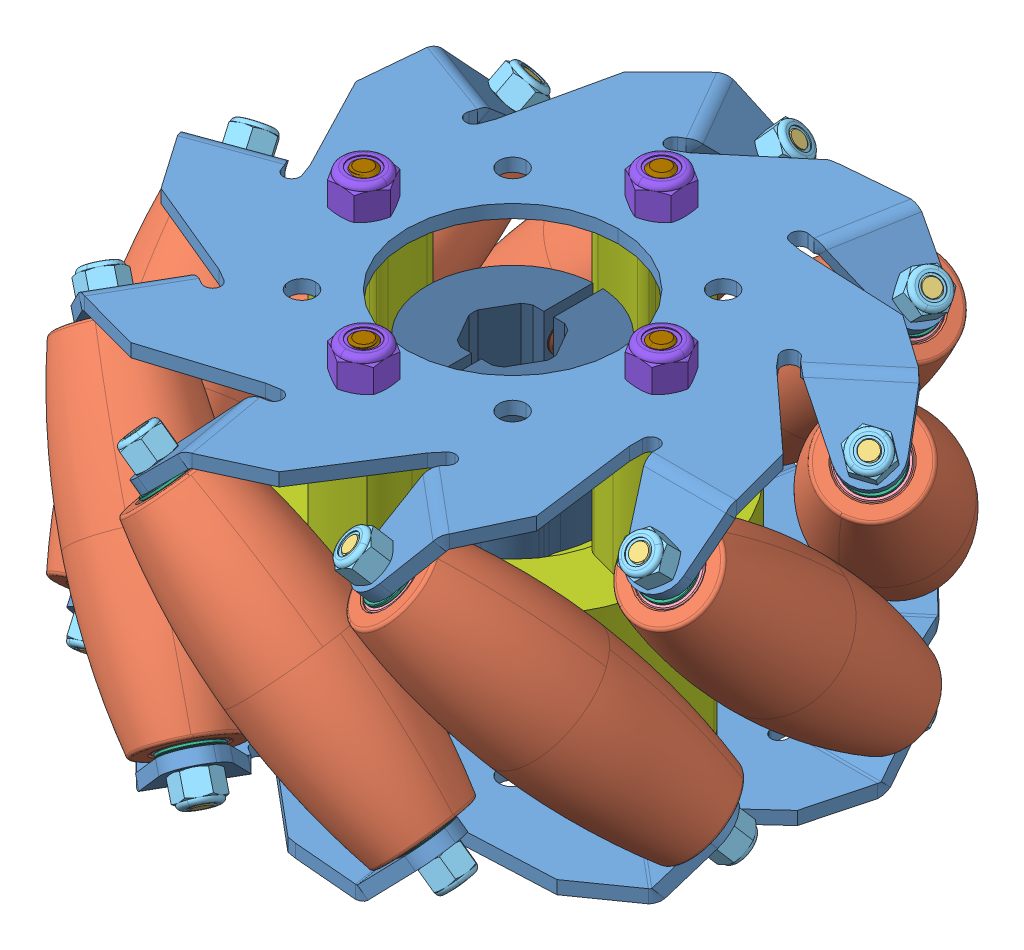
SolidWorks assembly Mecanum Right Slant With Hyper Hub, configuration Default. Lengths in mm.
Overall size (118.19 59.77 119.24).
88 component instances, 11 part files, 0 mates.
Components (placement in the parent):
- Mecanum 1.STEP-1: Mecanum 1.STEP [Default] at origin size (118.19 59.77 119.24)
  - 3606-0100-0100 Side Plate.STEP-1: 3606-0100-0100 Side Plate.STEP [Default] at (-29.0217 8.9207 26.0563) size (93.83 10.59 94.33)
  - 3606-0100-0100 Side Plate.STEP-2: 3606-0100-0100 Side Plate.STEP [Default] at (-29.0217 -77.2207 26.0563) x (1 0 0) z (0 0 -1) size (93.83 10.59 94.33)
  - 3606-XXXX-0100 Hi Durability Roller.STEP-1: 3606-XXXX-0100 Hi Durability Roller.STEP [Default] at (21.1711 -21.7418 81.2623) x (0.224554 0.052172 0.973064) z (0.696364 -0.707107 -0.122788) size (28.35 23.77 47)
  - 3606-XXXX-0100 Roller Axle.STEP-1: 3606-XXXX-0100 Roller Axle.STEP [Default] at (-21.9538 -34.2162 65.7074) x (0.715939 0.696364 0.050088) z (0.050088 -0.122788 0.991168) size (4 60.01 4)
  - 3606-XXXX-0100 Roller Bearing.STEP-1: 3606-XXXX-0100 Roller Bearing.STEP [Default] at (-35.5329 -20.4276 68.1018) x (0.715939 0.696364 0.050088) z (0.050088 -0.122788 0.991168) size (9 4 9)
  - 3606-XXXX-0100 Roller Locknut_90576A102.STEP-1: 3606-XXXX-0100 Roller Locknut_90576A102.STEP [Default] at (-40.1289 -15.7607 68.9122) x (0.353014 0.486435 -0.799226) z (0.624866 0.513207 0.588354) size (5.52 4.01 6.37)
  - 3606-XXXX-0100 Roller Shim.STEP-1: 3606-XXXX-0100 Roller Shim.STEP [Default] at (18.11 -15.3241 52.0807) x (0.434371 0.830389 -0.348965) z (-0.303693 0.499753 0.811183) size (7.84 5.87 6.18)
  - 3606-XXXX-0100 Wheel Center.STEP-1: 3606-XXXX-0100 Wheel Center.STEP [Default] at (-29.0217 -34.15 26.0563) x (-0.707107 0 0.707107) z (-0.707107 0 -0.707107) size (54 46 54)
  - 3606-XXXX-0100 Roller Bearing.STEP-2: 3606-XXXX-0100 Roller Bearing.STEP [Default] at (-8.514 -47.8634 63.3376) x (0.715939 0.696364 0.050088) z (-0.050088 0.122788 -0.991168) size (9 4 9)
  - 3606-XXXX-0100 Roller Shim.STEP-2: 3606-XXXX-0100 Roller Shim.STEP [Default] at (-6.4986 -109.4838 69.5446) x (-0.771195 -0.488369 0.408356) z (-0.621724 0.439939 -0.648007) size (7.84 5.87 6.18)
  - 3606-XXXX-0100 Roller Locknut_90576A102.STEP-2: 3606-XXXX-0100 Roller Locknut_90576A102.STEP [Default] at (-3.918 -52.5303 62.5272) x (-0.353014 -0.486435 0.799226) z (0.624866 0.513207 0.588354) size (5.52 4.01 6.37)
  - 3606-XXXX-0100 Roller Locknut_90576A102.STEP-3: 3606-XXXX-0100 Roller Locknut_90576A102.STEP [Default] at (-65.0776 -15.7607 51.7463) x (0.784157 0.486435 -0.38533) z (0.100489 0.513207 0.852362) size (5.52 4.01 6.37)
  - 3606-XXXX-0100 Roller Locknut_90576A102.STEP-4: 3606-XXXX-0100 Roller Locknut_90576A102.STEP [Default] at (-73.1553 -15.7607 22.5597) x (0.848384 0.486435 0.208867) z (-0.470909 0.513207 0.71754) size (5.52 4.01 6.37)
  - 3606-XXXX-0100 Roller Locknut_90576A102.STEP-5: 3606-XXXX-0100 Roller Locknut_90576A102.STEP [Default] at (-60.5824 -15.7607 -4.9907) x (0.515643 0.486435 0.705332) z (-0.821963 0.513207 0.246973) size (5.52 4.01 6.37)
  - 3606-XXXX-0100 Roller Locknut_90576A102.STEP-6: 3606-XXXX-0100 Roller Locknut_90576A102.STEP [Default] at (-33.242 -15.7607 -18.0139) x (-0.058373 0.486435 0.871765) z (-0.788411 0.513207 -0.339155) size (5.52 4.01 6.37)
  - 3606-XXXX-0100 Roller Locknut_90576A102.STEP-7: 3606-XXXX-0100 Roller Locknut_90576A102.STEP [Default] at (-3.9268 -15.7607 -10.4161) x (-0.605076 0.486435 0.630289) z (-0.385953 0.513207 -0.766589) size (5.52 4.01 6.37)
  - 3606-XXXX-0100 Roller Locknut_90576A102.STEP-8: 3606-XXXX-0100 Roller Locknut_90576A102.STEP [Default] at (13.6461 -15.7607 14.2475) x (-0.868657 0.486435 0.093894) z (0.197097 0.513207 -0.835327) size (5.52 4.01 6.37)
  - 3606-XXXX-0100 Roller Locknut_90576A102.STEP-9: 3606-XXXX-0100 Roller Locknut_90576A102.STEP [Default] at (11.2543 -15.7607 44.4366) x (-0.725784 0.486435 -0.486435) z (0.687923 0.513207 -0.513207) size (5.52 4.01 6.37)
  - 3606-XXXX-0100 Roller Locknut_90576A102.STEP-10: 3606-XXXX-0100 Roller Locknut_90576A102.STEP [Default] at (-9.9831 -15.7607 66.0254) x (-0.243308 0.486435 -0.839156) z (0.856862 0.513207 0.049049) size (5.52 4.01 6.37)
  - 3606-XXXX-0100 Roller Shim.STEP-3: 3606-XXXX-0100 Roller Shim.STEP [Default] at (-9.6449 -15.3241 76.2879) x (0.557058 0.830389 0.011885) z (-0.75406 0.499753 0.426192) size (7.84 5.87 6.18)
  - 3606-XXXX-0100 Roller Shim.STEP-4: 3606-XXXX-0100 Roller Shim.STEP [Default] at (-46.4664 -15.3241 76.9911) x (0.419091 0.830389 0.367174) z (-0.851595 0.499753 -0.158218) size (7.84 5.87 6.18)
  - 3606-XXXX-0100 Roller Shim.STEP-5: 3606-XXXX-0100 Roller Shim.STEP [Default] at (-75.1254 -15.3241 53.8614) x (0.085028 0.830389 0.550659) z (-0.550659 0.499753 -0.668597) size (7.84 5.87 6.18)
  - 3606-XXXX-0100 Roller Shim.STEP-6: 3606-XXXX-0100 Roller Shim.STEP [Default] at (-82.2119 -15.3241 17.7214) x (-0.288822 0.830389 0.476484) z (0.007937 0.499753 -0.866131) size (7.84 5.87 6.18)
  - 3606-XXXX-0100 Roller Shim.STEP-7: 3606-XXXX-0100 Roller Shim.STEP [Default] at (-64.4102 -15.3241 -14.5186) x (-0.527528 0.830389 0.179357) z (0.562818 0.499753 -0.658393) size (7.84 5.87 6.18)
  - 3606-XXXX-0100 Roller Shim.STEP-8: 3606-XXXX-0100 Roller Shim.STEP [Default] at (-30.0498 -15.3241 -27.7731) x (-0.519398 0.830389 -0.201693) z (0.854351 0.499753 -0.142586) size (7.84 5.87 6.18)
  - 3606-XXXX-0100 Roller Shim.STEP-9: 3606-XXXX-0100 Roller Shim.STEP [Default] at (4.7916 -15.3241 -15.8403) x (-0.268236 0.830389 -0.488369) z (0.746123 0.499753 0.439939) size (7.84 5.87 6.18)
  - 3606-XXXX-0100 Roller Shim.STEP-10: 3606-XXXX-0100 Roller Shim.STEP [Default] at (23.8114 -15.3241 15.6965) x (0.108437 0.830389 -0.546531) z (0.288776 0.499753 0.816612) size (7.84 5.87 6.18)
  - 3606-XXXX-0100 Roller Bearing.STEP-3: 3606-XXXX-0100 Roller Bearing.STEP [Default] at (-61.0359 -20.4276 54.0797) x (0.516245 0.696364 0.498566) z (-0.598741 -0.122788 0.791475) size (9 4 9)
  - 3606-XXXX-0100 Roller Bearing.STEP-4: 3606-XXXX-0100 Roller Bearing.STEP [Default] at (-71.5591 -20.4276 26.9452) x (0.074995 0.696364 0.71376) z (-0.967412 -0.122788 0.221441) size (9 4 9)
  - 3606-XXXX-0100 Roller Bearing.STEP-5: 3606-XXXX-0100 Roller Bearing.STEP [Default] at (-62.1786 -20.4276 -0.6053) x (-0.401347 0.696364 0.594977) z (-0.883421 -0.122788 -0.452207) size (9 4 9)
  - 3606-XXXX-0100 Roller Bearing.STEP-6: 3606-XXXX-0100 Roller Bearing.STEP [Default] at (-37.2836 -20.4276 -15.6804) x (-0.689893 0.696364 0.197798) z (-0.386067 -0.122788 -0.914262) size (9 4 9)
  - 3606-XXXX-0100 Roller Bearing.STEP-7: 3606-XXXX-0100 Roller Bearing.STEP [Default] at (-8.5228 -20.4276 -11.2265) x (-0.655631 0.696364 -0.291932) z (0.291932 -0.122788 -0.948524) size (9 4 9)
  - 3606-XXXX-0100 Roller Bearing.STEP-8: 3606-XXXX-0100 Roller Bearing.STEP [Default] at (10.6463 -20.4276 10.6724) x (-0.314592 0.696364 -0.645065) z (0.833333 -0.122788 -0.538961) size (9 4 9)
  - 3606-XXXX-0100 Roller Bearing.STEP-9: 3606-XXXX-0100 Roller Bearing.STEP [Default] at (11.2543 -20.4276 39.7697) x (0.173648 0.696364 -0.696364) z (0.984808 -0.122788 0.122788) size (9 4 9)
  - 3606-XXXX-0100 Roller Bearing.STEP-10: 3606-XXXX-0100 Roller Bearing.STEP [Default] at (-6.9833 -20.4276 62.4503) x (0.580637 0.696364 -0.421827) z (0.67548 -0.122788 0.727083) size (9 4 9)
  - 3606-XXXX-0100 Hi Durability Roller.STEP-2: 3606-XXXX-0100 Hi Durability Roller.STEP [Default] at (-26.0575 -21.7418 100.6099) x (-0.453455 0.052172 0.889751) z (0.612372 -0.707107 0.353553) size (28.35 23.77 47)
  - 3606-XXXX-0100 Hi Durability Roller.STEP-3: 3606-XXXX-0100 Hi Durability Roller.STEP [Default] at (-74.6731 -21.7418 85.073) x (-0.919288 0.052172 0.390113) z (0.241845 -0.707107 0.664463) size (28.35 23.77 47)
  - 3606-XXXX-0100 Hi Durability Roller.STEP-4: 3606-XXXX-0100 Hi Durability Roller.STEP [Default] at (-101.9279 -21.7418 41.9216) x (-0.954975 0.052172 -0.292062) z (-0.241845 -0.707107 0.664463) size (28.35 23.77 47)
  - 3606-XXXX-0100 Hi Durability Roller.STEP-5: 3606-XXXX-0100 Hi Durability Roller.STEP [Default] at (-95.0691 -21.7418 -8.6533) x (-0.543819 0.052172 -0.837579) z (-0.612372 -0.707107 0.353553) size (28.35 23.77 47)
  - 3606-XXXX-0100 Hi Durability Roller.STEP-6: 3606-XXXX-0100 Hi Durability Roller.STEP [Default] at (-57.306 -21.7418 -42.9873) x (0.121796 0.052172 -0.991183) z (-0.696364 -0.707107 -0.122788) size (28.35 23.77 47)
  - 3606-XXXX-0100 Hi Durability Roller.STEP-7: 3606-XXXX-0100 Hi Durability Roller.STEP [Default] at (-6.3084 -21.7418 -45.0149) x (0.730421 0.052172 -0.681002) z (-0.454519 -0.707107 -0.541675) size (28.35 23.77 47)
  - 3606-XXXX-0100 Hi Durability Roller.STEP-8: 3606-XXXX-0100 Hi Durability Roller.STEP [Default] at (34.0614 -21.7418 -13.7876) x (0.997274 0.052172 -0.052172) z (0 -0.707107 -0.707107) size (28.35 23.77 47)
  - 3606-XXXX-0100 Hi Durability Roller.STEP-9: 3606-XXXX-0100 Hi Durability Roller.STEP [Default] at (44.9139 -21.7418 36.0832) x (0.797492 0.052172 0.60107) z (0.454519 -0.707107 -0.541675) size (28.35 23.77 47)
  - 3606-XXXX-0100 Roller Bearing.STEP-11: 3606-XXXX-0100 Roller Bearing.STEP [Default] at (-37.2758 -47.8634 67.7976) x (0.516245 0.696364 0.498566) z (0.598741 0.122788 -0.791475) size (9 4 9)
  - 3606-XXXX-0100 Roller Bearing.STEP-12: 3606-XXXX-0100 Roller Bearing.STEP [Default] at (-62.1755 -47.8634 52.7264) x (0.074995 0.696364 0.71376) z (0.967412 0.122788 -0.221441) size (9 4 9)
  - 3606-XXXX-0100 Roller Bearing.STEP-13: 3606-XXXX-0100 Roller Bearing.STEP [Default] at (-71.5622 -47.8634 25.1759) x (-0.401347 0.696364 0.594977) z (0.883421 0.122788 0.452207) size (9 4 9)
  - 3606-XXXX-0100 Roller Bearing.STEP-14: 3606-XXXX-0100 Roller Bearing.STEP [Default] at (-61.0437 -47.8634 -1.9626) x (-0.689893 0.696364 0.197798) z (0.386067 0.122788 0.914262) size (9 4 9)
  - 3606-XXXX-0100 Roller Bearing.STEP-15: 3606-XXXX-0100 Roller Bearing.STEP [Default] at (-35.5418 -47.8634 -15.9907) x (-0.655631 0.696364 -0.291932) z (-0.291932 0.122788 0.948524) size (9 4 9)
  - 3606-XXXX-0100 Roller Bearing.STEP-16: 3606-XXXX-0100 Roller Bearing.STEP [Default] at (-6.989 -47.8634 -10.3446) x (-0.314592 0.696364 -0.645065) z (-0.833333 0.122788 0.538961) size (9 4 9)
  - 3606-XXXX-0100 Roller Bearing.STEP-17: 3606-XXXX-0100 Roller Bearing.STEP [Default] at (11.2543 -47.8634 12.334) x (0.173648 0.696364 -0.696364) z (-0.984808 0.122788 -0.122788) size (9 4 9)
  - 3606-XXXX-0100 Roller Bearing.STEP-18: 3606-XXXX-0100 Roller Bearing.STEP [Default] at (10.6521 -47.8634 41.4333) x (0.580637 0.696364 -0.421827) z (-0.67548 0.122788 -0.727083) size (9 4 9)
  - 3606-XXXX-0100 Roller Shim.STEP-11: 3606-XXXX-0100 Roller Shim.STEP [Default] at (-39.7217 -109.4838 73.8479) x (-0.853256 -0.488369 -0.182895) z (-0.059738 0.439939 -0.896038) size (7.84 5.87 6.18)
  - 3606-XXXX-0100 Roller Shim.STEP-12: 3606-XXXX-0100 Roller Shim.STEP [Default] at (-67.9382 -109.4838 55.789) x (-0.536069 -0.488369 -0.688568) z (0.530201 0.439939 -0.724804) size (7.84 5.87 6.18)
  - 3606-XXXX-0100 Roller Shim.STEP-13: 3606-XXXX-0100 Roller Shim.STEP [Default] at (-77.9453 -109.4838 23.8178) x (0.03195 -0.488369 -0.872052) z (0.872052 0.439939 -0.214425) size (7.84 5.87 6.18)
  - 3606-XXXX-0100 Roller Shim.STEP-14: 3606-XXXX-0100 Roller Shim.STEP [Default] at (-65.0604 -109.4838 -7.1059) x (0.58502 -0.488369 -0.647494) z (0.805861 0.439939 0.396285) size (7.84 5.87 6.18)
  - 3606-XXXX-0100 Roller Shim.STEP-15: 3606-XXXX-0100 Roller Shim.STEP [Default] at (-35.3127 -109.4838 -22.5127) x (0.864352 -0.488369 -0.119965) z (0.362598 0.439939 0.821569) size (7.84 5.87 6.18)
  - 3606-XXXX-0100 Roller Shim.STEP-16: 3606-XXXX-0100 Roller Shim.STEP [Default] at (-2.6213 -109.4838 -15.1934) x (0.739244 -0.488369 0.463696) z (-0.250328 0.439939 0.862432) size (7.84 5.87 6.18)
  - 3606-XXXX-0100 Roller Shim.STEP-17: 3606-XXXX-0100 Roller Shim.STEP [Default] at (17.717 -109.4838 11.427) x (0.268236 -0.488369 0.830389) z (-0.746123 0.439939 0.499753) size (7.84 5.87 6.18)
  - 3606-XXXX-0100 Roller Shim.STEP-18: 3606-XXXX-0100 Roller Shim.STEP [Default] at (16.1857 -109.4838 44.8927) x (-0.328283 -0.488369 0.808534) z (-0.892799 0.439939 -0.096765) size (7.84 5.87 6.18)
  - 3606-XXXX-0100 Roller Locknut_90576A102.STEP-11: 3606-XXXX-0100 Roller Locknut_90576A102.STEP [Default] at (-33.2342 -52.5303 70.1311) x (-0.784157 -0.486435 0.38533) z (0.100489 0.513207 0.852362) size (5.52 4.01 6.37)
  - 3606-XXXX-0100 Roller Locknut_90576A102.STEP-12: 3606-XXXX-0100 Roller Locknut_90576A102.STEP [Default] at (-60.5793 -52.5303 57.1118) x (-0.848384 -0.486435 -0.208867) z (-0.470909 0.513207 0.71754) size (5.52 4.01 6.37)
  - 3606-XXXX-0100 Roller Locknut_90576A102.STEP-13: 3606-XXXX-0100 Roller Locknut_90576A102.STEP [Default] at (-73.1583 -52.5303 29.5614) x (-0.515643 -0.486435 -0.705332) z (-0.821963 0.513207 0.246973) size (5.52 4.01 6.37)
  - 3606-XXXX-0100 Roller Locknut_90576A102.STEP-14: 3606-XXXX-0100 Roller Locknut_90576A102.STEP [Default] at (-65.0853 -52.5303 0.3709) x (0.058373 -0.486435 -0.871765) z (-0.788411 0.513207 -0.339155) size (5.52 4.01 6.37)
  - 3606-XXXX-0100 Roller Locknut_90576A102.STEP-15: 3606-XXXX-0100 Roller Locknut_90576A102.STEP [Default] at (-40.1378 -52.5303 -16.8011) x (0.605076 -0.486435 -0.630289) z (-0.385953 0.513207 -0.766589) size (5.52 4.01 6.37)
  - 3606-XXXX-0100 Roller Locknut_90576A102.STEP-16: 3606-XXXX-0100 Roller Locknut_90576A102.STEP [Default] at (-9.9889 -52.5303 -13.9196) x (0.868657 -0.486435 -0.093894) z (0.197097 0.513207 -0.835327) size (5.52 4.01 6.37)
  - 3606-XXXX-0100 Roller Locknut_90576A102.STEP-17: 3606-XXXX-0100 Roller Locknut_90576A102.STEP [Default] at (11.2543 -52.5303 7.6671) x (0.725784 -0.486435 0.486435) z (0.687923 0.513207 -0.513207) size (5.52 4.01 6.37)
  - 3606-XXXX-0100 Roller Locknut_90576A102.STEP-18: 3606-XXXX-0100 Roller Locknut_90576A102.STEP [Default] at (13.6519 -52.5303 37.8583) x (0.243308 -0.486435 0.839156) z (0.856862 0.513207 0.049049) size (5.52 4.01 6.37)
  - 3606-XXXX-0100 Roller Axle.STEP-2: 3606-XXXX-0100 Roller Axle.STEP [Default] at (-49.0946 -34.2162 60.974) x (0.516245 0.696364 0.498566) z (-0.598741 -0.122788 0.791475) size (4 60.01 4)
  - 3606-XXXX-0100 Roller Axle.STEP-3: 3606-XXXX-0100 Roller Axle.STEP [Default] at (-66.8431 -34.2162 39.9022) x (0.074995 0.696364 0.71376) z (-0.967412 -0.122788 0.221441) size (4 60.01 4)
  - 3606-XXXX-0100 Roller Axle.STEP-4: 3606-XXXX-0100 Roller Axle.STEP [Default] at (-66.8946 -34.2162 12.3518) x (-0.401347 0.696364 0.594977) z (-0.883421 -0.122788 -0.452207) size (4 60.01 4)
  - 3606-XXXX-0100 Roller Axle.STEP-5: 3606-XXXX-0100 Roller Axle.STEP [Default] at (-49.2249 -34.2162 -8.7862) x (-0.689893 0.696364 0.197798) z (-0.386067 -0.122788 -0.914262) size (4 60.01 4)
  - 3606-XXXX-0100 Roller Axle.STEP-6: 3606-XXXX-0100 Roller Axle.STEP [Default] at (-22.1019 -34.2162 -13.6209) x (-0.655631 0.696364 -0.291932) z (0.291932 -0.122788 -0.948524) size (4 60.01 4)
  - 3606-XXXX-0100 Roller Axle.STEP-7: 3606-XXXX-0100 Roller Axle.STEP [Default] at (1.7832 -34.2162 0.1098) x (-0.314592 0.696364 -0.645065) z (0.833333 -0.122788 -0.538961) size (4 60.01 4)
  - 3606-XXXX-0100 Roller Axle.STEP-8: 3606-XXXX-0100 Roller Axle.STEP [Default] at (11.2543 -34.2162 25.9811) x (0.173648 0.696364 -0.696364) z (0.984808 -0.122788 0.122788) size (4 60.01 4)
  - 3606-XXXX-0100 Roller Axle.STEP-9: 3606-XXXX-0100 Roller Axle.STEP [Default] at (1.8799 -34.2162 51.8877) x (0.580637 0.696364 -0.421827) z (0.67548 -0.122788 0.727083) size (4 60.01 4)
  - 2812-0004-0007_90576A103.STEP-1: 2812-0004-0007_90576A103.STEP [Default] at (-29.0217 -9.15 3.4289) size (7.02 4.86 8.1)
  - 2800-0004-0055_90128A207.STEP-1: 2800-0004-0055_90128A207.STEP [Default] at (-29.0217 -4.15 3.4289) x (1 0 0) z (0 1 0) size (9.08 9.66 59.77)
  - 2800-0004-0055_90128A207.STEP-2: 2800-0004-0055_90128A207.STEP [Default] at (-6.3943 -4.15 26.0563) x (0 0 1) z (0 1 0) size (9.08 9.66 59.77)
  - 2800-0004-0055_90128A207.STEP-3: 2800-0004-0055_90128A207.STEP [Default] at (-29.0217 -4.15 48.6837) x (-1 0 0) z (0 1 0) size (9.08 9.66 59.77)
  - 2800-0004-0055_90128A207.STEP-4: 2800-0004-0055_90128A207.STEP [Default] at (-51.6491 -4.15 26.0563) x (0 0 -1) z (0 1 0) size (9.08 9.66 59.77)
  - 2812-0004-0007_90576A103.STEP-2: 2812-0004-0007_90576A103.STEP [Default] at (-6.3943 -9.15 26.0563) x (0 0 1) z (-1 0 0) size (7.02 4.86 8.1)
  - 2812-0004-0007_90576A103.STEP-3: 2812-0004-0007_90576A103.STEP [Default] at (-29.0217 -9.15 48.6837) x (-1 0 0) z (0 0 -1) size (7.02 4.86 8.1)
  - 2812-0004-0007_90576A103.STEP-4: 2812-0004-0007_90576A103.STEP [Default] at (-51.6491 -9.15 26.0563) x (0 0 -1) z (1 0 0) size (7.02 4.86 8.1)
- 12mm Hyper Hub.STEP-2: 12mm Hyper Hub.STEP [Default] at (-21.2546 -43.5502 7.9551) x (-1 0 0) z (0 1 0) size (26 26 21)
  - 1310-0016-4012.STEP-1: 1310-0016-4012.STEP [Default] at (7.7672 18.1012 8.4002) size (26 26 21)
  - 2800-0004-0014_90128A207.STEP-1: 2800-0004-0014_90128A207.STEP [Default] at (-1.9828 25.8512 24.0002) x (0 0 1) z (-1 0 0) size (7 7 18.01)
  - 2800-0004-0014_90128A207.STEP-2: 2800-0004-0014_90128A207.STEP [Default] at (17.5172 10.3512 24.0002) x (0 0 1) z (1 0 0) size (7 7 18.01)
